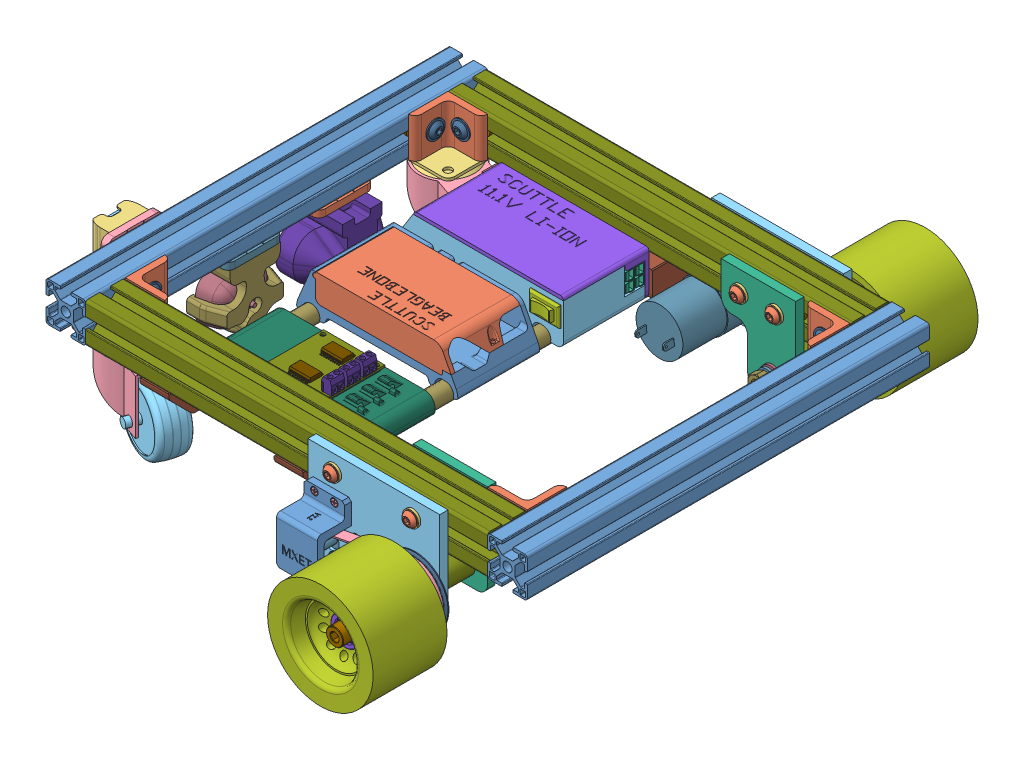
SolidWorks assembly FullRobot, configuration Default. Lengths in mm.
Overall size (385.75 100.57 463.5).
206 component instances, 66 part files, 26 mates.
Components (placement in the parent):
- Chassis-1: Chassis [Default] at origin size (364.8 100.57 305.12)
  - tSlot 30mm-1: tSlot 30mm [5537T736] at origin size (30 30 304.8)
  - tSlot 30mm-5: tSlot 30mm [5537T736] at (334.7999 0 0) size (30 30 304.8)
  - bracket30mm-1: bracket30mm [5537T936] at (14.9999 -0.0001 -122.4) x (1 0 0) z (0 -1 0) size (30 30 30)
  - bracket30mm-2: bracket30mm [5537T936] at (14.9999 0.0001 122.4) x (1 0 0) z (0 1 0) size (30 30 30)
  - bracket30mm-4: bracket30mm [5537T936] at (319.7999 -0.0001 122.4) x (0 0 -1) z (0 1 0) size (30 30 30)
  - bracket30mm-6: bracket30mm [5537T936] at (319.7999 -0.0001 -122.4) x (-1 0 0) z (0 1 0) size (30 30 30)
  - caster-1: caster [Default] at (-27.5104 -55.7119 137.6001) x (0 0 -1) z (1 0 0) size (61.73 78.47 82.51)
    - Caster_2_1-1: Caster_2_1 [Default] at (18.5848 38.712 45.8952) size (50 10.47 50)
    - caster_2_2-1: caster_2_2 [Default] at (18.5848 -9.7561 45.8952) x (0.329712 0 -0.944081) z (0.944081 0 0.329712) size (53 41 44)
    - caster_2_3-1: caster_2_3 [Default] at (2.9227 -3.7561 65.8469) x (0.329629 0.022474 -0.943843) z (0.00741 -0.999747 -0.021218) size (51.07 40 51.07)
    - fastener-1: fastener [Default] at (0.2 32.912 27.5104) x (-0.837169 0 -0.546944) z (0 -1 0) size (11.8 11.81 15.93)
      - Screw M6x10mm-1: Screw M6x10mm [91352A141] at origin size (10.5 10.5 13.87)
      - washer, lock M6-1: washer, lock M6 [92148A180] at (0 0 -4.8) size (11.8 11.81 3.22)
      - Nut M6-1: Nut M6 [91828A251] at (0 0 -12.8) size (10 11.55 5.57)
    - fastener-4: fastener [Default] at (36.9696 32.912 27.5104) x (-0.295217 0 -0.95543) z (0 -1 0) size (11.8 11.81 15.93)
      - Screw M6x10mm-1: Screw M6x10mm [91352A141] at origin size (10.5 10.5 13.87)
      - washer, lock M6-1: washer, lock M6 [92148A180] at (0 0 -4.8) size (11.8 11.81 3.22)
      - Nut M6-1: Nut M6 [91828A251] at (0 0 -12.8) size (10 11.55 5.57)
  - caster-2: caster [Default] at (-27.5104 -55.7119 -100.4095) x (0 0 -1) z (1 0 0) size (61.73 78.47 82.51)
    - Caster_2_1-1: Caster_2_1 [Default] at (18.5848 38.712 45.8952) size (50 10.47 50)
    - caster_2_2-1: caster_2_2 [Default] at (18.5848 -9.7561 45.8952) x (0.329712 0 -0.944081) z (0.944081 0 0.329712) size (53 41 44)
    - caster_2_3-1: caster_2_3 [Default] at (2.9227 -3.7561 65.8469) x (0.329629 0.022474 -0.943843) z (0.00741 -0.999747 -0.021218) size (51.07 40 51.07)
    - fastener-1: fastener [Default] at (0.2 32.912 27.5104) x (-0.837169 0 -0.546944) z (0 -1 0) size (11.8 11.81 15.93)
      - Screw M6x10mm-1: Screw M6x10mm [91352A141] at origin size (10.5 10.5 13.87)
      - washer, lock M6-1: washer, lock M6 [92148A180] at (0 0 -4.8) size (11.8 11.81 3.22)
      - Nut M6-1: Nut M6 [91828A251] at (0 0 -12.8) size (10 11.55 5.57)
    - fastener-4: fastener [Default] at (36.9696 32.912 27.5104) x (-0.295217 0 -0.95543) z (0 -1 0) size (11.8 11.81 15.93)
      - Screw M6x10mm-1: Screw M6x10mm [91352A141] at origin size (10.5 10.5 13.87)
      - washer, lock M6-1: washer, lock M6 [92148A180] at (0 0 -4.8) size (11.8 11.81 3.22)
      - Nut M6-1: Nut M6 [91828A251] at (0 0 -12.8) size (10 11.55 5.57)
  - TSlotFastener_chassis-1: TSlotFastener_chassis [Default] at (17.3335 -0.0001 -107.4) x (0 0 -1) z (0 -1 0) size (25.4 16.7 15.56)
    - t slot fastener-1: t slot fastener [Default] at origin size (25.4 3.15 11.25)
    - t slot screw-1: t slot screw [Default] at (0 2.6664 0) x (0.991402 0 -0.130855) z (0.130855 0 0.991402) size (13.87 16.7 13.87)
  - TSlotFastener_chassis-2: TSlotFastener_chassis [Default] at (17.3335 0.0001 107.4) x (0 0 -1) z (0 -1 0) size (25.4 16.7 15.56)
    - t slot fastener-1: t slot fastener [Default] at origin size (25.4 3.15 11.25)
    - t slot screw-1: t slot screw [Default] at (0 2.6664 0) x (0.991402 0 -0.130855) z (0.130855 0 0.991402) size (13.87 16.7 13.87)
  - TSlotFastener_chassis-4: TSlotFastener_chassis [Default] at (317.4664 -0.0001 107.4) x (0 0 1) z (0 -1 0) size (25.4 16.7 15.56)
    - t slot fastener-1: t slot fastener [Default] at origin size (25.4 3.15 11.25)
    - t slot screw-1: t slot screw [Default] at (0 2.6664 0) x (0.991402 0 -0.130855) z (0.130855 0 0.991402) size (13.87 16.7 13.87)
  - TSlotFastener_chassis-7: TSlotFastener_chassis [Default] at (317.4664 -0.0001 -107.4) x (0 0 1) z (0 -1 0) size (25.4 16.7 15.56)
    - t slot fastener-1: t slot fastener [Default] at origin size (25.4 3.15 11.25)
    - t slot screw-1: t slot screw [Default] at (0 2.6664 0) x (0.991402 0 -0.130855) z (0.130855 0 0.991402) size (13.87 16.7 13.87)
  - TSlotFastener_chassis-8: TSlotFastener_chassis [Default] at (304.7999 -0.0001 -120.0664) x (1 0 0) z (0 -1 0) size (25.4 16.7 15.56)
    - t slot fastener-1: t slot fastener [Default] at origin size (25.4 3.15 11.25)
    - t slot screw-1: t slot screw [Default] at (0 2.6664 0) x (0.991402 0 -0.130855) z (0.130855 0 0.991402) size (13.87 16.7 13.87)
  - TSlotFastener_chassis-9: TSlotFastener_chassis [Default] at (304.7999 -0.0001 120.0664) x (-1 0 0) z (0 -1 0) size (25.4 16.7 15.56)
    - t slot fastener-1: t slot fastener [Default] at origin size (25.4 3.15 11.25)
    - t slot screw-1: t slot screw [Default] at (0 2.6664 0) x (0.991402 0 -0.130855) z (0.130855 0 0.991402) size (13.87 16.7 13.87)
  - TSlotFastener_chassis-10: TSlotFastener_chassis [Default] at (29.9999 -0.0001 -120.0664) x (1 0 0) z (0 -1 0) size (25.4 16.7 15.56)
    - t slot fastener-1: t slot fastener [Default] at origin size (25.4 3.15 11.25)
    - t slot screw-1: t slot screw [Default] at (0 2.6664 0) x (0.991402 0 -0.130855) z (0.130855 0 0.991402) size (13.87 16.7 13.87)
  - TSlotFastener_chassis-11: TSlotFastener_chassis [Default] at (29.9999 0.0001 120.0664) x (-1 0 0) z (0 -1 0) size (25.4 16.7 15.56)
    - t slot fastener-1: t slot fastener [Default] at origin size (25.4 3.15 11.25)
    - t slot screw-1: t slot screw [Default] at (0 2.6664 0) x (0.991402 0 -0.130855) z (0.130855 0 0.991402) size (13.87 16.7 13.87)
  - fastener-1: fastener [Default] at (36.7696 -22.7999 -137.3791) x (1 0 0) z (0 -1 0) size (11.8 11.81 15.93)
    - Screw M6x10mm-1: Screw M6x10mm [91352A141] at origin size (10.5 10.5 13.87)
    - washer, lock M6-1: washer, lock M6 [92148A180] at (0 0 -4.8) size (11.8 11.81 3.22)
    - Nut M6-1: Nut M6 [91828A251] at (0 0 -12.8) size (10 11.55 5.57)
  - fastener-2: fastener [Default] at (36.7696 -22.7999 137.4001) x (1 0 0) z (0 -1 0) size (11.8 11.81 15.93)
    - Screw M6x10mm-1: Screw M6x10mm [91352A141] at origin size (10.5 10.5 13.87)
    - washer, lock M6-1: washer, lock M6 [92148A180] at (0 0 -4.8) size (11.8 11.81 3.22)
    - Nut M6-1: Nut M6 [91828A251] at (0 0 -12.8) size (10 11.55 5.57)
- RailLg-1: RailLg [Default] at (179.7999 -5.6347 137.4001) x (0 0 -1) z (-1 0 0) size (304.8 36.47 129.1)
  - ShaftBracketLg V2-1: ShaftBracketLg V2 [Default] at origin size (40 30.97 22)
  - ShaftBracketLg V2-2: ShaftBracketLg V2 [Default] at (0 0 101.6) size (40 30.97 22)
  - tubeLg-1: tubeLg [Default] at (136.8249 21.1653 11) x (0 -0.883839 -0.467791) z (1 0 0) size (12.7 12.7 247.65)
  - tubeLg-2: tubeLg [Default] at (136.8249 21.1653 112.6) x (0 -0.961886 -0.273452) z (1 0 0) size (12.7 12.7 247.65)
  - ShaftBracketLg V2-3: ShaftBracketLg V2 [Default] at (274.8 0 22) x (-1 0 0) z (0 0 -1) size (40 30.97 22)
  - ShaftBracketLg V2-6: ShaftBracketLg V2 [Default] at (274.8 0 123.6) x (-1 0 0) z (0 0 -1) size (40 30.97 22)
  - rodSecure-1: rodSecure [Default] at (269.8001 9.3653 112.35) x (0 0 1) z (-1 0 0) size (33.5 27.3 20)
- DriveTrainRight-1: DriveTrainRight [Default] at (284.7999 -56.0001 -158.7499) size (304.8 98 143.85)
  - Motor-1-1: Motor-1 [Default] at (-83.0905 19.8847 62.85) x (-0.996341 -0.085462 0) z (0 0 -1) size (37 37 84)
  - flat head screw-1: flat head screw [Default] at (-89.8737 28.3251 0) x (0.999225 0.039359 0) z (0 0 -1) size (6 6 10.3)
  - flat head screw-2: flat head screw [Default] at (-63.4348 23.6632 0) x (0.923728 0.383049 0) z (0 0 -1) size (6 6 10.3)
  - flat head screw-3: flat head screw [Default] at (-80.6915 3.0974 0) x (-0.923728 -0.383049 0) z (0 0 -1) size (6 6 10.3)
  - 30mm rail-1: 30mm rail [Default] at (-117.4 56.0001 21.3499) x (0 0 1) z (-1 0 0) size (30 30 304.8)
  - small pulley-1-1: small pulley-1 [Default] at (-82.5 14 -6.5) x (0 0 -1) z (1 0 0) size (15 28 28)
  - encoder-1: encoder [Default] at (-88.97 13 -20.75) x (0 1 0) z (0 0 1) size (21.9 28.1 10.4)
  - encoderBracketV2-1: encoderBracketV2 [Default] at (-98 1 0) x (0 0 -1) z (1 0 0) size (25.75 47 31.28)
  - AssemTSlotScrew-1: AssemTSlotScrew [Default] at (-41.75 56 40.4424) x (1 0 0) z (0 -1 0) size (25.4 17.89 14.53)
    - t slot fastener-1: t slot fastener [Default] at origin size (25.4 3.15 11.25)
    - M6x14mm Screw-1: M6x14mm Screw [91239A319] at (0 7.75 0) x (-0.837169 0 -0.546944) z (0 1 0) size (10.5 10.5 17.89)
    - M6 Flat Washer-1: M6 Flat Washer [93475A250] at (0 2.65 0) x (1 0 0) z (0 1 0) size (12 12 1.8)
  - AssemTSlotScrew-2: AssemTSlotScrew [Default] at (-14.75 56 40.4424) x (1 0 0) z (0 -1 0) size (25.4 17.89 14.53)
    - t slot fastener-1: t slot fastener [Default] at origin size (25.4 3.15 11.25)
    - M6x14mm Screw-1: M6x14mm Screw [91239A319] at (0 7.75 0) x (-0.837169 0 -0.546944) z (0 1 0) size (10.5 10.5 17.89)
    - M6 Flat Washer-1: M6 Flat Washer [93475A250] at (0 2.65 0) x (1 0 0) z (0 1 0) size (12 12 1.8)
  - AssemTSlotScrew-3: AssemTSlotScrew [Default] at (-80 58.3 2.2575) x (-1 0 0) z (0 -1 0) size (25.4 17.89 14.53)
    - t slot fastener-1: t slot fastener [Default] at origin size (25.4 3.15 11.25)
    - M6x14mm Screw-1: M6x14mm Screw [91239A319] at (0 7.75 0) x (-0.837169 0 -0.546944) z (0 1 0) size (10.5 10.5 17.89)
    - M6 Flat Washer-1: M6 Flat Washer [93475A250] at (0 2.65 0) x (1 0 0) z (0 1 0) size (12 12 1.8)
  - AssemTSlotScrew-4: AssemTSlotScrew [Default] at (-20 58.3 2.2575) x (-1 0 0) z (0 -1 0) size (25.4 17.89 14.53)
    - t slot fastener-1: t slot fastener [Default] at origin size (25.4 3.15 11.25)
    - M6x14mm Screw-1: M6x14mm Screw [91239A319] at (0 7.75 0) x (-0.837169 0 -0.546944) z (0 1 0) size (10.5 10.5 17.89)
    - M6 Flat Washer-1: M6 Flat Washer [93475A250] at (0 2.65 0) x (1 0 0) z (0 1 0) size (12 12 1.8)
  - Screw M2.5x10 92010A020-1: Screw M2.5x10 92010A020 [92010A020] at (-75 44 -3.5) x (-1 0 0) z (0 0 -1) size (4.7 4.7 10.19)
  - Screw M2.5x10 92010A020-2: Screw M2.5x10 92010A020 [92010A020] at (-90 44 -3.5) x (-1 0 0) z (0 0 -1) size (4.7 4.7 10.19)
  - plate1-1: plate1 [Default] at (-100 -1 0) size (100 72 6.35)
  - plate2v3-1: plate2v3 [Default] at (0 -1 36.3499) size (56.5 72 6.35)
  - AssemWheel-1: AssemWheel [Default] at (-17.5 13 -35.6628) x (1 0 0) z (0 -1 0) size (80 129.21 80)
    - wheel V1-1: wheel V1 [Default] at origin size (80 56 80)
    - ballBearing608 v1-1: ballBearing608 v1 [5972K91] at (0 2.1628 0) x (0 0 -1) z (0 -1 0) size (22 22 7)
    - ballBearing608 v1-2: ballBearing608 v1 [5972K91] at (0 -15.0872 0) x (0 0 -1) z (0 -1 0) size (22 22 7)
    - Screw M8x110mm-1: Screw M8x110mm [Default] at (0 91.4128 0) x (0 0 1) z (0 1 0) size (13 13 118.81)
    - wheel Pulley v1-1: wheel Pulley v1 [Default] at (0 24.1628 0) x (0 1 0) z (0 0 1) size (48.5 51 51)
    - Spacer, bearing v1-1: Spacer, bearing v1 [Default] at (0 -11.5872 0) x (1 0 0) z (0 1 0) size (10.13 10.13 10.25)
    - M8 hex nut-1-1: M8 hex nut-1 [Default] at (0 87.4033 0) x (1 0 0) z (0 -1 0) size (13 15.01 7.38)
    - Washer M8, Flat-1: Washer M8, Flat [93475A270] at (0 78.3628 0) x (0.931601 0 0.363483) z (0 1 0) size (16 16 1.8)
    - Washer, M8 lock-1: Washer, M8 lock [92148A200] at (0 82.0628 0) x (0.935203 0 -0.354113) z (0 -1 0) size (15.56 14.81 4.08)
    - shaft sleeve V1-1: shaft sleeve V1 [Default] at (0 5.6628 0) x (1 0 0) z (0 1 0) size (16 16 30)
    - shaft spacer V1-1: shaft spacer V1 [Default] at (0 42.0128 0) x (1 0 0) z (0 1 0) size (16 16 30)
- UltraSonic-1: UltraSonic [Default] at (27 -49.6999 -45.4502) x (0 0 -1) z (-1 0 0) size (65 59.92 42)
  - ultrasonicBracket-1: ultrasonicBracket [Default] at origin size (65 45.75 35.19)
  - Sensor Ultrasonic v2-1: Sensor Ultrasonic v2 [Default] at (0 0 22.85) size (45.42 26.14 17.7)
  - Socket-1: Socket [Header] at (-3.8375 -17.5389 17.475) size (2.5 14.1 2.5)
  - universal V2.1-1: universal V2.1 [Default] at (11 -43.3653 27) x (0 0 1) z (-1 0 0) size (30 19.17 42)
- DriveTrainLeft-1: DriveTrainLeft [Default] at (167.3999 0 137.4001) x (0 0 -1) z (1 0 0) size (143.85 98 304.8)
  - plate1-1: plate1 [Default] at (-14.9999 -57.0001 22.4) x (0 0 1) z (-1 0 0) size (100 72 6.35)
  - Motor-1-1: Motor-1 [Default] at (41.5001 -36.1153 39.3095) x (0 0.085462 0.996341) z (-1 0 0) size (37 37 84)
  - flat head screw-1: flat head screw [Default] at (-21.3499 -27.6749 32.5263) x (0 0.221945 -0.975059) z (-1 0 0) size (6 6 10.3)
  - flat head screw-2: flat head screw [Default] at (-21.3499 -32.3368 58.9652) x (0 -0.373736 0.927535) z (-1 0 0) size (6 6 10.3)
  - flat head screw-4: flat head screw [Default] at (-21.3499 -52.9027 41.7085) x (0 -0.567989 0.823036) z (-1 0 0) size (6 6 10.3)
  - AssemTSlotScrew-1: AssemTSlotScrew [Default] at (-19.0925 3.2999 42.4) x (0 0 1) z (0 -1 0) size (25.4 17.89 14.53)
    - t slot fastener-1: t slot fastener [Default] at origin size (25.4 3.15 11.25)
    - M6x14mm Screw-1: M6x14mm Screw [91239A319] at (0 7.75 0) x (-0.837169 0 -0.546944) z (0 1 0) size (10.5 10.5 17.89)
    - M6 Flat Washer-1: M6 Flat Washer [93475A250] at (0 2.65 0) x (1 0 0) z (0 1 0) size (12 12 1.8)
  - AssemTSlotScrew-2: AssemTSlotScrew [Default] at (-19.0925 3.2999 102.4) x (0 0 1) z (0 -1 0) size (25.4 17.89 14.53)
    - t slot fastener-1: t slot fastener [Default] at origin size (25.4 3.15 11.25)
    - M6x14mm Screw-1: M6x14mm Screw [91239A319] at (0 7.75 0) x (-0.837169 0 -0.546944) z (0 1 0) size (10.5 10.5 17.89)
    - M6 Flat Washer-1: M6 Flat Washer [93475A250] at (0 2.65 0) x (1 0 0) z (0 1 0) size (12 12 1.8)
  - 30mm rail-1: 30mm rail [Default] at origin size (30 30 304.8)
  - small pulley-1-1: small pulley-1 [Default] at (-26.8499 -43.0001 39.9) x (-1 0 0) z (0 0.194011 -0.980999) size (15 28 28) (hidden)
  - encoder-1: encoder [Default] at (-41.0999 -43.0001 33.43) x (0 -1 0) z (1 0 0) size (21.9 28.1 10.4)
  - encoderBracketV2-1: encoderBracketV2 [Default] at (-21.3499 -55.0001 55.4) x (-1 0 0) z (0 0 -1) size (25.75 47 31.28)
  - AssemTSlotScrew-6: AssemTSlotScrew [Default] at (19.0925 -0.0001 107.65) x (0 0 1) z (0 1 0) size (25.4 17.89 14.53)
    - t slot fastener-1: t slot fastener [Default] at origin size (25.4 3.15 11.25)
    - M6x14mm Screw-1: M6x14mm Screw [91239A319] at (0 7.75 0) x (-0.837169 0 -0.546944) z (0 1 0) size (10.5 10.5 17.89)
    - M6 Flat Washer-1: M6 Flat Washer [93475A250] at (0 2.65 0) x (1 0 0) z (0 1 0) size (12 12 1.8)
  - AssemTSlotScrew-8: AssemTSlotScrew [Default] at (19.0925 -0.0001 80.65) x (0 0 1) z (0 1 0) size (25.4 17.89 14.53)
    - t slot fastener-1: t slot fastener [Default] at origin size (25.4 3.15 11.25)
    - M6x14mm Screw-1: M6x14mm Screw [91239A319] at (0 7.75 0) x (-0.837169 0 -0.546944) z (0 1 0) size (10.5 10.5 17.89)
    - M6 Flat Washer-1: M6 Flat Washer [93475A250] at (0 2.65 0) x (1 0 0) z (0 1 0) size (12 12 1.8)
  - Screw No.0 92470A018-1: Screw No.0 92470A018 [92470A018] at (-39.3499 -33.9251 34.32) x (0 0 -1) z (1 0 0) size (2.95 2.95 5.82)
  - Screw No.0 92470A018-2: Screw No.0 92470A018 [92470A018] at (-39.3499 -52.0751 45.48) x (0 0.158553 -0.987351) z (1 0 0) size (2.95 2.95 5.82)
  - Screw M2.5x10 92010A020-1: Screw M2.5x10 92010A020 [92010A020] at (-24.8499 -12.0001 32.4) x (0 0 1) z (-1 0 0) size (4.7 4.7 10.19)
  - Screw M2.5x10 92010A020-2: Screw M2.5x10 92010A020 [92010A020] at (-24.8499 -12.0001 47.4) x (0 0 1) z (-1 0 0) size (4.7 4.7 10.19)
  - belt-1: belt [Default] at (-25.0999 -43.0001 104.9) x (0 0 -1) z (-1 0 0) size (101.91 48.76 8)
  - plate2v3-1: plate2v3 [Default] at (21.3499 -57.0001 122.4) x (0 0 1) z (-1 0 0) size (56.5 72 6.35)
  - AssemWheel-1: AssemWheel [Default] at (-57.0127 -43.0001 104.9) x (0 0 -1) z (0 -1 0) size (80 129.21 80)
    - wheel V1-1: wheel V1 [Default] at origin size (80 56 80)
    - ballBearing608 v1-1: ballBearing608 v1 [5972K91] at (0 2.1628 0) x (0 0 -1) z (0 -1 0) size (22 22 7)
    - ballBearing608 v1-2: ballBearing608 v1 [5972K91] at (0 -15.0872 0) x (0 0 -1) z (0 -1 0) size (22 22 7)
    - Screw M8x110mm-1: Screw M8x110mm [Default] at (0 91.4128 0) x (0 0 1) z (0 1 0) size (13 13 118.81)
    - wheel Pulley v1-1: wheel Pulley v1 [Default] at (0 24.1628 0) x (0 1 0) z (0 0 1) size (48.5 51 51)
    - Spacer, bearing v1-1: Spacer, bearing v1 [Default] at (0 -11.5872 0) x (1 0 0) z (0 1 0) size (10.13 10.13 10.25)
    - M8 hex nut-1-1: M8 hex nut-1 [Default] at (0 87.4033 0) x (1 0 0) z (0 -1 0) size (13 15.01 7.38)
    - Washer M8, Flat-1: Washer M8, Flat [93475A270] at (0 78.3628 0) x (0.931601 0 0.363483) z (0 1 0) size (16 16 1.8)
    - Washer, M8 lock-1: Washer, M8 lock [92148A200] at (0 82.0628 0) x (0.935203 0 -0.354113) z (0 -1 0) size (15.56 14.81 4.08)
    - shaft sleeve V1-1: shaft sleeve V1 [Default] at (0 5.6628 0) x (1 0 0) z (0 1 0) size (16 16 30)
    - shaft spacer V1-1: shaft spacer V1 [Default] at (0 42.0128 0) x (1 0 0) z (0 1 0) size (16 16 30)
- BatteryPack-1: BatteryPack [Default] at (155.9499 0.3001 -105.1263) x (-1 0 0) z (0 1 0) size (127 69.85 34.5)
  - batteryHolderV3-1: batteryHolderV3 [Default] at origin size (127 65 32)
  - AssemPowerPoles-1: AssemPowerPoles [Default] at (-6.0899 7.3277 -12.9633) x (0 0 -1) z (-1 0 0) size (20.55 17 29.35)
    - powerpolePP75-1: powerpolePP75 [Rouge] at origin size (8.15 8.15 21.4)
    - powerpolePP75-2: powerpolePP75 [Rouge] at (-7.7103 0 0) size (8.15 8.15 21.4)
    - powerpolePP75-3: powerpolePP75 [Rouge] at (0 -7.7103 0) size (8.15 8.15 21.4)
    - powerpolePP75-4: powerpolePP75 [Rouge] at (-7.7103 -7.7103 0) size (8.15 8.15 21.4)
    - ppShroud-1: ppShroud [Default] at (-4.0633 4.4641 14.4562) x (1 0 0) z (0 -1 0) size (20.55 22.15 17) (hidden)
  - switchSRB22-1: switchSRB22 [Default] at (-24.9992 65 -15.6541) size (23.06 25.63 15.01)
  - lidV2-2: lidV2 [Default] at (-28.75 65 5.5) x (1 0 0) z (0 0 -1) size (119.25 65 31.5)
  - 3cellPack-1: 3cellPack [Default] at (73.8009 -15.3584 -29.3812) x (1 0 0) z (0 -1 0) size (77.72 24.8 62)
    - battery3cell-1: battery3cell [Default] at (-33.4129 6.5562 -47.5134) size (77.72 24.77 59.69)
    - 18650 battery-1: 18650 battery [Default] at (-66.783 8.6095 -83.6496) x (1 0 0) z (0 -0.187564 0.982252) size (65 18 18)
    - 18650 battery-2: 18650 battery [Default] at (-66.783 11.4552 -65.3283) x (1 0 0) z (0 -0.34093 0.940089) size (65 18 18)
    - 18650 battery-3: 18650 battery [Default] at (-66.783 13.8247 -46.2326) x (1 0 0) z (0 -0.457859 0.889025) size (65 18 18)
  - Screw M2.5x8-1: Screw M2.5x8 [92010A018] at (84.75 1.5 -12.1) x (0.837169 0 0.546944) z (0 -1 0) size (4.7 4.7 8.17)
  - Screw M2.5x8-2: Screw M2.5x8 [92010A018] at (-21.75 1.5 -22) x (0.925243 0 0.379375) z (0 -1 0) size (4.7 4.7 8.17)
- Camera-1: Camera [Default] at (14.5 -53.1999 23.2513) x (0 0 -1) z (-1 0 0) size (53 68.17 30)
  - cameraShell v2-1: cameraShell v2 [Default] at origin size (53 54 25.5)
  - MicrosoftCamera-1: MicrosoftCamera [Default] at (0 0 5.3) size (44.33 37.25 25.5)
  - universal V2.1-cam-1: universal V2.1-cam [Default] at (11 -46.8653 14.5) x (0 0 1) z (-1 0 0) size (30 19.17 42)
- MotorDriver-1: MotorDriver [Default] at (179.7999 -15.2999 52.2739) x (-1 0 0) z (0 0 1) size (122 25 48)
  - DualMotorDriverMount-1: DualMotorDriverMount [Default] at origin size (122 17.4 48)
  - driverHW231-1: driverHW231 [Default] at (61 0 24) x (0 0 1) z (0 -1 0) size (47.4 46.77 14.5)
    - MotorDriverHW321-1: MotorDriverHW321 [Default] at origin size (47.4 46.3 1.6)
    - ScrewTerminal-1: ScrewTerminal [Default] at (-1.6863 28.0693 0.1876) x (1 0 0) z (0 -1 0) size (10.29 14.5 7.6)
    - ScrewTerminal-2: ScrewTerminal [Default] at (-13.9363 28.0693 0.1876) x (1 0 0) z (0 -1 0) size (10.29 14.5 7.6)
    - ScrewTerminal-3: ScrewTerminal [Default] at (10.5637 28.0693 0.1876) x (1 0 0) z (0 -1 0) size (10.29 14.5 7.6)
    - ScrewTerminal-4: ScrewTerminal [Default] at (-1.6863 28.0693 0.1876) x (1 0 0) z (0 -1 0) size (10.29 14.5 7.6)
    - SO20-3: SO20 [Default] at (-12.2 -1.045 1.6) size (12.87 15.81 3.23)
    - SO20-4: SO20 [Default] at (12.2 -1.045 1.6) x (-1 0 0) z (0 0 1) size (12.87 15.81 3.23)
- beagleBone-1: beagleBone [Default] at (119.032 0.8639 11.7468) x (-1 0 0) z (0 0 -1) size (122.2 33 64.82)
  - BeagleMount V2.1-1: BeagleMount V2.1 [Default] at (1.8321 -27.6639 -21.7625) size (122.2 31 62)
  - PcbCover-1: PcbCover [Default] at (-56.2274 -19.0639 -21.7625) size (104.8 20.5 59)
  - BeagleBoard-1: BeagleBoard [Default] at (5.0921 -22.5639 9.4325) size (89.96 17.2 54.61) (hidden)
    - BBBlue_PCB-1: BBBlue_PCB [Default] at (-43.12 8.5 27.305) size (86.36 13.32 54.61)
    - PJ-102B_12V_PWRJACK-1: PJ-102B_12V_PWRJACK [Default] at (-46.12 16.6 -21.605) x (-1 0 0) z (0 0 -1) size (14.4 14.5 9.4)
    - USB1-1: USB1 [Default] at (-39.2199 13.516 19.2088) x (0 0 -1) z (1 0 0) size (14.3 10.22 14.65)
    - MicroUSB1-1: MicroUSB1 [Default] at (-44.12 6.6 -14.805) x (1 0 0) z (0 -1 0) size (5.31 7.52 3.41)
    - pin-header-8x3-1: pin-header-8x3 [Default] at (25.24 13.3281 -21.6059) x (1 0 0) z (0 -0.112945 -0.993601) size (7.62 13.38 20.48)
  - Rpi3Bplus-1: Rpi3Bplus [Default] at (46.1821 -14.0639 -22.1125) x (-1 0 0) z (0 0 -1) size (87.03 17.52 58.47) (hidden)
- compass-1: compass [Default] at (-18.8499 15 83.9141) x (0 0 1) z (0 -1 0) size (42 29.42 30)
  - compassClip v2-1: compassClip v2 [Default] at origin size (30 15.25 21)
  - universal bracket V2.1-1: universal bracket V2.1 [Default] at (11 -12.5153 15) x (0 0 1) z (-1 0 0) size (30 19.17 42)
  - pmod cmps-1: pmod cmps [Default] at (0 13.15 11.8) x (1 0 0) z (0 1 0) size (20.6 20.6 1.5)
Mates (geometry in assembly coordinates):
- Coincident8: coincident aligned: plane of Chassis-1/tSlot 30mm-1 through (0 0 0) normal (0 1 0); plane of assembly through (0 0 0) normal (0 1 0)
- Coincident9: coincident aligned: plane of Chassis-1/tSlot 30mm-1 through (0 0 0) normal (1 0 0); plane of assembly through (0 0 0) normal (1 0 0)
- Coincident10: coincident aligned: plane of Chassis-1/tSlot 30mm-1 through (0 0 0) normal (0 0 1); plane of assembly through (0 0 0) normal (0 0 1)
- Coincident11: coincident aligned: plane of RailLg-1/ShaftBracketLg V2-1; plane of assembly through (0 0 137.4001) normal (0 0 1)
- Coincident17: coincident anti-aligned: plane of Chassis-1/bracket30mm-1 through (44.9999 -15.0001 -122.4) normal (0 0 -1); plane of DriveTrainRight-1/30mm rail-1 through (14.9999 4.5 -122.4) normal (0 0 1)
- Coincident18: coincident: line of Chassis-1/bracket30mm-1 through (14.9999 -15.0001 -122.4) axis (0 1 0); plane of DriveTrainRight-1/30mm rail-1 through (14.9999 -4.5 -122.9) normal (-1 0 0)
- Coincident19: coincident aligned: plane of Chassis-1/tSlot 30mm-1 through (12.9999 14.9999 152.4) normal (0 1 0); plane of DriveTrainRight-1/30mm rail-1 through (14.9999 14.9999 -124.4) normal (0 1 0)
- Coincident23: coincident aligned: plane of Chassis-1/tSlot 30mm-1 through (14.4999 -4.5 152.4) normal (0 0 1); plane of DriveTrainLeft-1/30mm rail-1 through (319.7999 12.9999 152.4) normal (0 0 1)
- Coincident24: coincident aligned: plane of Chassis-1/tSlot 30mm-1 through (12.9999 14.9999 152.4) normal (0 1 0); plane of DriveTrainLeft-1/30mm rail-1 through (319.7999 14.9999 124.4001) normal (0 1 0)
- Coincident25: coincident anti-aligned: plane of Chassis-1/tSlot 30mm-1 through (14.9999 4.5 152.4) normal (1 0 0); plane of DriveTrainLeft-1/30mm rail-1 through (14.9999 -4.5 122.9001) normal (-1 0 0)
- Concentric5: concentric anti-aligned: cylinder of BatteryPack-1/batteryHolderV3-1 through (67.1999 -26.7999 -40.1263) axis (0 0 -1) radius 6.5; cylinder of RailLg-1/tubeLg-2 through (67.1999 -26.7999 -123.2499) axis (0 0 1) radius 6.35
- Parallel4: parallel aligned: plane of BatteryPack-1/batteryHolderV3-1 through (155.9499 0.3001 -105.1263) normal (0 1 0); plane of assembly through (0 0 0) normal (0 1 0)
- Coincident28: coincident anti-aligned: plane of Chassis-1/tSlot 30mm-1 through (0 0 0) normal (1 0 0); plane of ? through (0 -1.6228 -64.8536) normal (-1 0 0)
- Coincident29: coincident anti-aligned: plane of Chassis-1/tSlot 30mm-1 through (4.5 12.7425 152.4) normal (0 -1 0); plane of ? through (-9 12.7425 -80.8536) normal (0 1 0)
- Coincident30: coincident anti-aligned: plane of RailLg-1/ShaftBracketLg V2-2 through (56.1999 -14.9999 141.9001) normal (0 1 0); plane of DriveTrainLeft-1/30mm rail-1 through (319.7999 -14.9999 150.4) normal (0 -1 0)
- Distance4: distance = 10 mm anti-aligned: plane of RailLg-1/ShaftBracketLg V2-1 through (179.7999 -14.2999 132.9001) normal (1 0 0); plane of DriveTrainLeft-1/plate1-1 through (189.7999 -57.0001 158.75) normal (-1 0 0)
- Parallel6: parallel anti-aligned: plane of MotorDriver-1/DualMotorDriverMount-1; plane of assembly through (0 0 0) normal (0 1 0)
- Concentric8: concentric aligned: cylinder of RailLg-1/tubeLg-2 through (67.1999 -26.7999 -123.2499) axis (0 0 1) radius 6.35; cylinder of beagleBone-1/BeagleMount V2.1-1 through (67.1999 -26.7999 -28.4906) axis (0 0 1) radius 6.5
- Parallel7: parallel aligned: plane of beagleBone-1; plane of assembly through (0 0 0) normal (0 1 0)
- Coincident31: coincident anti-aligned: plane of Chassis-1/tSlot 30mm-1 through (0 0 0) normal (0 1 0); plane of compass-1/compassClip v2-1 through (-18.8499 0 83.9141) normal (0 -1 0)
- Coincident32: coincident anti-aligned: plane of Chassis-1/tSlot 30mm-1 through (-14.9999 -4.5 152.4) normal (-1 0 0); plane of compass-1/universal bracket V2.1-1 through (-14.9999 -4 62.9141) normal (1 0 0)
- Coincident33: coincident anti-aligned: plane of Chassis-1/tSlot 30mm-1 through (-12.9999 -14.9999 152.4) normal (0 -1 0); plane of UltraSonic-1/universal V2.1-1 through (-4 -14.9999 -66.4502) normal (0 1 0)
- Coincident34: coincident anti-aligned: plane of Chassis-1/tSlot 30mm-1 through (0 0 0) normal (1 0 0); plane of UltraSonic-1/universal V2.1-1
- Coincident35: coincident anti-aligned: plane of Chassis-1/tSlot 30mm-1 through (-12.9999 -14.9999 152.4) normal (0 -1 0); plane of Camera-1/cameraShell v2-1
- Coincident36: coincident anti-aligned: plane of Chassis-1/tSlot 30mm-1 through (0 0 0) normal (1 0 0); plane of Camera-1/cameraShell v2-1 through (0 -53.1999 23.2513) normal (-1 0 0)
- Concentric9: concentric anti-aligned: cylinder of RailLg-1/tubeLg-1 through (168.7999 -26.7999 -123.2499) axis (0 0 1) radius 6.35; circle of MotorDriver-1/DualMotorDriverMount-1
